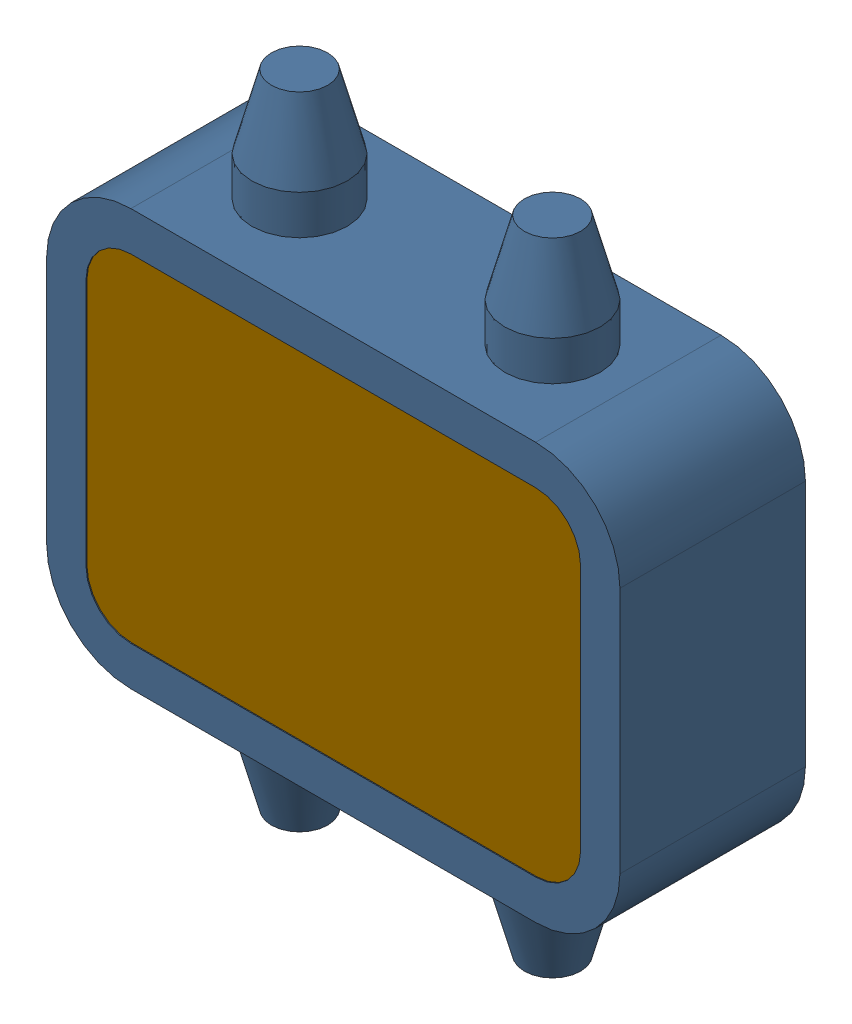
SolidWorks assembly boitier_ordinateur, configuration Défaut. Lengths in mm.
Overall size (204 228 66).
11 component instances, 10 part files, 0 mates.
Components (placement in the parent):
- raspberryPi3B-1: raspberryPi3B [Detailed] at (124.9064 268.957 66.7989) x (0 -1 0) z (0 0 1) size (87.05 58.5 19.05)
- Copie de RockBLOCK_9603^boitier_ordinateur-1: Copie de RockBLOCK_9603^boitier_ordinateur [Défaut] at (19.3394 271.6927 69.6398) x (-1 0 0) z (0 1 0) size (45.05 17 54.85) (virtual)
  - RockBLOCK V 3B^Copie de RockBLOCK_9603_boitier_ordinateur-1: RockBLOCK V 3B^Copie de RockBLOCK_9603_boitier_ordinateur [Défaut] at origin size (31.5 10.6 29.6) (virtual)
  - RockBLOCK V 3B-0^Copie de RockBLOCK_9603_boitier_ordinateur-1: RockBLOCK V 3B-0^Copie de RockBLOCK_9603_boitier_ordinateur [Défaut] at origin size (5.5 2.4 5.5) (virtual)
  - RockBLOCK V 3B-1^Copie de RockBLOCK_9603_boitier_ordinateur-1: RockBLOCK V 3B-1^Copie de RockBLOCK_9603_boitier_ordinateur [Défaut] at origin size (5.5 2.4 5.5) (virtual)
  - RockBLOCK V 3B-2^Copie de RockBLOCK_9603_boitier_ordinateur-1: RockBLOCK V 3B-2^Copie de RockBLOCK_9603_boitier_ordinateur [Défaut] at origin size (45.05 17 54.85) (virtual)
- Copie de HU-10^boitier_ordinateur-1: Copie de HU-10^boitier_ordinateur [Défaut] at (32.1939 249.2373 80.6053) x (0 1 0) z (0 0 -1) size (13.03 3.05 6.6) (virtual)
- Copie de HU-6^boitier_ordinateur-1: Copie de HU-6^boitier_ordinateur [Défaut] at (102.8811 265.8631 77.1806) x (0 -1 0) z (-1 0 0) size (8.9 11.37 67.92) (virtual)
- NAVIO2-1: NAVIO2 [Predeterminado] at (124.8025 279.0319 75.8341) x (0 1 0) z (1 0 0) size (73.82 8.2 56.43)
- Copie de 300070_2^boitier_ordinateur-1: Copie de 300070_2^boitier_ordinateur [Défaut] at (70.4117 270.6146 101.2998) x (-1 0 0) z (0 0 -1) size (196 140 15) (virtual)
- Copie de 300070_1^boitier_ordinateur-1: Copie de 300070_1^boitier_ordinateur [Défaut] at (70.4117 270.6146 50.1134) size (204 228 66) (virtual)
